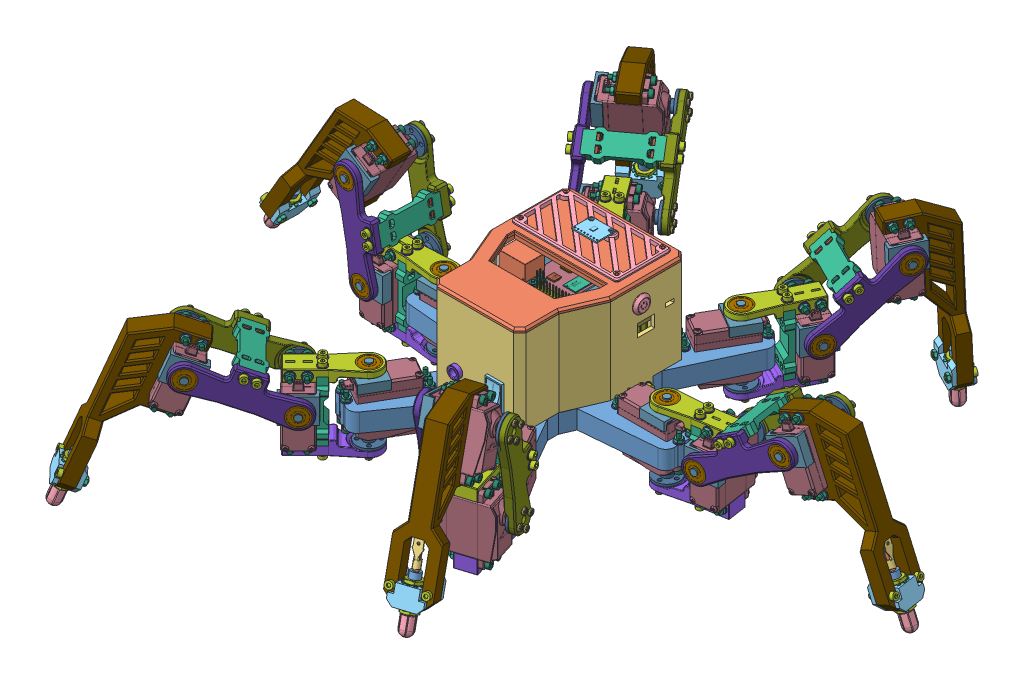
SolidWorks assembly HEXUMI_DSSERVO, configuration Default. Lengths in mm. (continued)
Mates (geometry in assembly coordinates): (continued)
- Concentric24: concentric aligned: cylinder of M3_WASHER-16 through (-104.9 0.5 30.3) axis (0 -1 0) radius 1.6; cylinder of M3_HEX_NUT-23 through (-104.9 2.9 30.3) axis (0 -1 0) radius 1.5
- Concentric25: concentric aligned: cylinder of M3_WASHER-15 through (-55.3 0.5 20.3) axis (0 -1 0) radius 1.6; cylinder of M3_HEX_NUT-20 through (-55.3 2.9 20.3) axis (0 -1 0) radius 1.5
- Coincident21: coincident anti-aligned: plane of M3_WASHER-15 through (-55.3 0.5 20.3) normal (0 1 0); plane of M3_HEX_NUT-20 through (-55.3 0.5 20.3) normal (0 -1 0)
- Coincident22: coincident anti-aligned: plane of M3_WASHER-17 through (-66.6069 0.5 -80.2666) normal (0 1 0); plane of M3_HEX_NUT-22 through (-66.6069 0.5 -80.2666) normal (0 -1 0)
- Coincident23: coincident anti-aligned: plane of M3_WASHER-16 through (-104.9 0.5 30.3) normal (0 1 0); plane of M3_HEX_NUT-23 through (-104.9 0.5 30.3) normal (0 -1 0)
- Concentric26: concentric aligned: circle of M3_WASHER-13; circle of M3_HEX_NUT-16
- Coincident24: coincident anti-aligned: plane of M3_WASHER-13 through (-33.1467 0.5 -42.3117) normal (0 1 0); plane of M3_HEX_NUT-16 through (-33.1467 0.5 -42.3117) normal (0 -1 0)
- Coincident25: coincident anti-aligned: plane of M3_WASHER-11 through (-41.8069 0.5 -37.3117) normal (0 1 0); plane of M3_HEX_NUT-10 through (-41.8069 0.5 -37.3117) normal (0 -1 0)
- Coincident26: coincident anti-aligned: plane of M3_WASHER-12 through (-57.9467 0.5 -85.2666) normal (0 1 0); plane of M3_HEX_NUT-21 through (-57.9467 0.5 -85.2666) normal (0 -1 0)
- Coincident27: coincident anti-aligned: plane of M3_WASHER-14 through (-55.3 0.5 30.3) normal (0 1 0); plane of M3_HEX_NUT-19 through (-55.3 0.5 30.3) normal (0 -1 0)
- Coincident29: coincident anti-aligned: plane of M3_WASHER-8 through (-66.9533 0.5 131.0666) normal (0 1 0); plane of M3_HEX_NUT-9 through (-66.9533 0.5 131.0666) normal (0 -1 0)
- Coincident30: coincident anti-aligned: plane of M3_WASHER-9 through (33.1467 0.5 -42.3117) normal (0 1 0); plane of M3_HEX_NUT-8 through (33.1467 0.5 -42.3117) normal (0 -1 0)
- Coincident31: coincident anti-aligned: plane of M3_WASHER-5 through (41.8069 0.5 -37.3117) normal (0 1 0); plane of M3_HEX_NUT-14 through (41.8069 0.5 -37.3117) normal (0 -1 0)
- Coincident32: coincident anti-aligned: plane of M3_WASHER-6 through (-42.1533 0.5 88.1117) normal (0 1 0); plane of M3_HEX_NUT-15 through (-42.1533 0.5 88.1117) normal (0 -1 0)
- Coincident33: coincident anti-aligned: plane of M3_WASHER-1 through (-58.2931 0.5 136.0666) normal (0 1 0); plane of M3_HEX_NUT-24 through (-58.2931 0.5 136.0666) normal (0 -1 0)
- Coincident34: coincident anti-aligned: plane of M3_WASHER-23 through (66.6069 0.5 -80.2666) normal (0 1 0); plane of M3_HEX_NUT-18 through (66.6069 0.5 -80.2666) normal (0 -1 0)
- Coincident35: coincident anti-aligned: plane of M3_WASHER-22 through (57.9467 0.5 -85.2666) normal (0 1 0); plane of M3_HEX_NUT-11 through (57.9467 0.5 -85.2666) normal (0 -1 0)
- Coincident36: coincident anti-aligned: plane of M3_WASHER-21 through (58.2931 0.5 136.0666) normal (0 1 0); plane of M3_HEX_NUT-4 through (58.2931 0.5 136.0666) normal (0 -1 0)
- Coincident37: coincident anti-aligned: plane of M3_WASHER-20 through (66.9533 0.5 131.0666) normal (0 1 0); plane of M3_HEX_NUT-17 through (66.9533 0.5 131.0666) normal (0 -1 0)
- Coincident38: coincident anti-aligned: plane of M3_WASHER-18 through (104.9 0.5 20.3) normal (0 1 0); plane of M3_HEX_NUT-2 through (104.9 0.5 20.3) normal (0 -1 0)
- Coincident39: coincident anti-aligned: plane of M3_WASHER-19 through (33.4931 0.5 93.1117) normal (0 1 0); plane of M3_HEX_NUT-3 through (33.4931 0.5 93.1117) normal (0 -1 0)
- Coincident40: coincident anti-aligned: plane of M3_WASHER-7 through (55.3 0.5 30.3) normal (0 1 0); plane of M3_HEX_NUT-7 through (55.3 0.5 30.3) normal (0 -1 0)
- Coincident41: coincident anti-aligned: plane of M3_WASHER-2 through (42.1533 0.5 88.1117) normal (0 1 0); plane of M3_HEX_NUT-5 through (42.1533 0.5 88.1117) normal (0 -1 0)
- Coincident42: coincident anti-aligned: plane of M3_WASHER-3 through (104.9 0.5 30.3) normal (0 1 0); plane of M3_HEX_NUT-6 through (104.9 0.5 30.3) normal (0 -1 0)
- Coincident43: coincident anti-aligned: plane of M3_WASHER-4 through (55.3 0.5 20.3) normal (0 1 0); plane of M3_HEX_NUT-13 through (55.3 0.5 20.3) normal (0 -1 0)
- Coincident44: coincident anti-aligned: plane of M3_WASHER-10 through (-33.4931 0.5 93.1117) normal (0 1 0); plane of M3_HEX_NUT-12 through (-33.4931 0.5 93.1117) normal (0 -1 0)
- Concentric27: concentric aligned: cylinder of BODY_ASM-1/MAIN_FRAME-1 through (-104.9 0 30.3) axis (0 -1 0) radius 1.5; cylinder of M3_STEEL_HEX_BOLT-20 through (-104.9 6.8 30.3) axis (0 -1 0) radius 1.5
- Concentric28: concentric aligned: cylinder of BODY_ASM-1/MAIN_FRAME-1 through (-104.9 0 20.3) axis (0 -1 0) radius 1.5; cylinder of M3_STEEL_HEX_BOLT-19 through (-104.9 6.8 20.3) axis (0 -1 0) radius 1.5
- Concentric29: concentric aligned: cylinder of BODY_ASM-1/MAIN_FRAME-1 through (-57.9467 0 -85.2666) axis (0 -1 0) radius 1.5; cylinder of M3_STEEL_HEX_BOLT-18 through (-57.9467 6.8 -85.2666) axis (0 -1 0) radius 1.5
- Concentric30: concentric aligned: cylinder of BODY_ASM-1/MAIN_FRAME-1 through (-66.6069 0 -80.2666) axis (0 -1 0) radius 1.5; cylinder of M3_STEEL_HEX_BOLT-17 through (-66.6069 6.8 -80.2666) axis (0 -1 0) radius 1.5
- Concentric31: concentric aligned: cylinder of BODY_ASM-1/MAIN_FRAME-1 through (57.9467 0 -85.2666) axis (0 -1 0) radius 1.5; cylinder of M3_STEEL_HEX_BOLT-16 through (57.9467 6.8 -85.2666) axis (0 -1 0) radius 1.5
- Concentric32: concentric aligned: cylinder of BODY_ASM-1/MAIN_FRAME-1 through (66.6069 0 -80.2666) axis (0 -1 0) radius 1.5; cylinder of M3_STEEL_HEX_BOLT-15 through (66.6069 6.8 -80.2666) axis (0 -1 0) radius 1.5
- Concentric33: concentric aligned: cylinder of BODY_ASM-1/MAIN_FRAME-1 through (104.9 0 30.3) axis (0 -1 0) radius 1.5; cylinder of M3_STEEL_HEX_BOLT-2 through (104.9 6.8 30.3) axis (0 -1 0) radius 1.5
- Concentric34: concentric aligned: cylinder of BODY_ASM-1/MAIN_FRAME-1 through (104.9 0 20.3) axis (0 -1 0) radius 1.5; cylinder of M3_STEEL_HEX_BOLT-14 through (104.9 6.8 20.3) axis (0 -1 0) radius 1.5
- Concentric35: concentric aligned: cylinder of BODY_ASM-1/MAIN_FRAME-1 through (66.9533 0 131.0666) axis (0 -1 0) radius 1.5; cylinder of M3_STEEL_HEX_BOLT-1 through (66.9533 6.8 131.0666) axis (0 -1 0) radius 1.5
- Concentric36: concentric aligned: cylinder of BODY_ASM-1/MAIN_FRAME-1 through (58.2931 0 136.0666) axis (0 -1 0) radius 1.5; cylinder of M3_STEEL_HEX_BOLT-24 through (58.2931 6.8 136.0666) axis (0 -1 0) radius 1.5
- Concentric37: concentric aligned: cylinder of BODY_ASM-1/MAIN_FRAME-1 through (-58.2931 0 136.0666) axis (0 -1 0) radius 1.5; cylinder of M3_STEEL_HEX_BOLT-3 through (-58.2931 6.8 136.0666) axis (0 -1 0) radius 1.5
- Concentric38: concentric aligned: cylinder of BODY_ASM-1/MAIN_FRAME-1 through (-66.9533 0 131.0666) axis (0 -1 0) radius 1.5; cylinder of M3_STEEL_HEX_BOLT-21 through (-66.9533 6.8 131.0666) axis (0 -1 0) radius 1.5
- Concentric39: concentric aligned: cylinder of BODY_ASM-1/MAIN_FRAME-1 through (-42.1533 0 88.1117) axis (0 -1 0) radius 1.5; cylinder of M3_STEEL_HEX_BOLT-13 through (-42.1533 6.8 88.1117) axis (0 -1 0) radius 1.5
- Concentric40: concentric aligned: cylinder of BODY_ASM-1/MAIN_FRAME-1 through (-33.4931 0 93.1117) axis (0 -1 0) radius 1.5; cylinder of M3_STEEL_HEX_BOLT-12 through (-33.4931 6.8 93.1117) axis (0 -1 0) radius 1.5
- Concentric41: concentric aligned: cylinder of BODY_ASM-1/MAIN_FRAME-1 through (-55.3 0 30.3) axis (0 -1 0) radius 1.5; cylinder of M3_STEEL_HEX_BOLT-11 through (-55.3 6.8 30.3) axis (0 -1 0) radius 1.5
- Concentric42: concentric aligned: cylinder of BODY_ASM-1/MAIN_FRAME-1 through (-55.3 0 20.3) axis (0 -1 0) radius 1.5; cylinder of M3_STEEL_HEX_BOLT-10 through (-55.3 6.8 20.3) axis (0 -1 0) radius 1.5
- Concentric43: concentric aligned: cylinder of BODY_ASM-1/MAIN_FRAME-1 through (33.4931 0 93.1117) axis (0 -1 0) radius 1.5; cylinder of M3_STEEL_HEX_BOLT-9 through (33.4931 6.8 93.1117) axis (0 -1 0) radius 1.5
- Concentric44: concentric aligned: cylinder of BODY_ASM-1/MAIN_FRAME-1 through (42.1533 0 88.1117) axis (0 -1 0) radius 1.5; cylinder of M3_STEEL_HEX_BOLT-8 through (42.1533 6.8 88.1117) axis (0 -1 0) radius 1.5
- Concentric45: concentric aligned: cylinder of BODY_ASM-1/MAIN_FRAME-1 through (55.3 0 30.3) axis (0 -1 0) radius 1.5; cylinder of M3_STEEL_HEX_BOLT-7 through (55.3 6.8 30.3) axis (0 -1 0) radius 1.5
- Concentric46: concentric aligned: cylinder of BODY_ASM-1/MAIN_FRAME-1 through (55.3 0 20.3) axis (0 -1 0) radius 1.5; cylinder of M3_STEEL_HEX_BOLT-6 through (55.3 6.8 20.3) axis (0 -1 0) radius 1.5
- Concentric47: concentric aligned: cylinder of BODY_ASM-1/MAIN_FRAME-1 through (41.8069 0 -37.3117) axis (0 -1 0) radius 1.5; cylinder of M3_STEEL_HEX_BOLT-5 through (41.8069 6.8 -37.3117) axis (0 -1 0) radius 1.5
- Concentric48: concentric aligned: cylinder of BODY_ASM-1/MAIN_FRAME-1 through (33.1467 0 -42.3117) axis (0 -1 0) radius 1.5; cylinder of M3_STEEL_HEX_BOLT-23 through (33.1467 6.8 -42.3117) axis (0 -1 0) radius 1.5
- Concentric49: concentric aligned: cylinder of BODY_ASM-1/MAIN_FRAME-1 through (-33.1467 0 -42.3117) axis (0 -1 0) radius 1.5; cylinder of M3_STEEL_HEX_BOLT-22 through (-33.1467 6.8 -42.3117) axis (0 -1 0) radius 1.5
- Concentric50: concentric aligned: cylinder of BODY_ASM-1/MAIN_FRAME-1 through (-41.8069 0 -37.3117) axis (0 -1 0) radius 1.5; cylinder of M3_STEEL_HEX_BOLT-4 through (-41.8069 6.8 -37.3117) axis (0 -1 0) radius 1.5
- Coincident46: coincident anti-aligned: plane of LEG_L-1/SERVO_ASM-2/SW2020 DS3225MG Servo 25Kg 4.8-6.8V-2 through (-54.8768 -18.2 -69.9494) normal (0 -1 0); plane of M3_STEEL_HEX_BOLT-4 through (-41.8069 -18.2 -37.3117) normal (0 1 0)
- Coincident47: coincident anti-aligned: plane of LEG_L-1/SERVO_ASM-2/SW2020 DS3225MG Servo 25Kg 4.8-6.8V-2 through (-54.8768 -18.2 -69.9494) normal (0 -1 0); plane of M3_STEEL_HEX_BOLT-22 through (-33.1467 -18.2 -42.3117) normal (0 1 0)
- Coincident48: coincident anti-aligned: plane of LEG_L-3/SERVO_ASM-2/SW2020 DS3225MG Servo 25Kg 4.8-6.8V-2 through (-90.1 -18.2 25.3) normal (0 -1 0); plane of M3_STEEL_HEX_BOLT-10 through (-55.3 -18.2 20.3) normal (0 1 0)
- Coincident49: coincident anti-aligned: plane of LEG_L-1/SERVO_ASM-2/SW2020 DS3225MG Servo 25Kg 4.8-6.8V-2 through (-54.8768 -18.2 -69.9494) normal (0 -1 0); plane of M3_STEEL_HEX_BOLT-18 through (-57.9467 -18.2 -85.2666) normal (0 1 0)
- Coincident50: coincident anti-aligned: plane of LEG_L-1/SERVO_ASM-2/SW2020 DS3225MG Servo 25Kg 4.8-6.8V-2 through (-54.8768 -18.2 -69.9494) normal (0 -1 0); plane of M3_STEEL_HEX_BOLT-17 through (-66.6069 -18.2 -80.2666) normal (0 1 0)
- Coincident51: coincident anti-aligned: plane of LEG_L-3/SERVO_ASM-2/SW2020 DS3225MG Servo 25Kg 4.8-6.8V-2 through (-90.1 -18.2 25.3) normal (0 -1 0); plane of M3_STEEL_HEX_BOLT-20 through (-104.9 -18.2 30.3) normal (0 1 0)
- Coincident52: coincident anti-aligned: plane of LEG_L-3/SERVO_ASM-2/SW2020 DS3225MG Servo 25Kg 4.8-6.8V-2 through (-90.1 -18.2 25.3) normal (0 -1 0); plane of M3_STEEL_HEX_BOLT-19 through (-104.9 -18.2 20.3) normal (0 1 0)
- Coincident53: coincident anti-aligned: plane of LEG_L-2/SERVO_ASM-2/SW2020 DS3225MG Servo 25Kg 4.8-6.8V-2 through (-55.2232 -18.2 120.7494) normal (0 -1 0); plane of M3_STEEL_HEX_BOLT-3 through (-58.2931 -18.2 136.0666) normal (0 1 0)
- Coincident54: coincident anti-aligned: plane of LEG_L-2/SERVO_ASM-2/SW2020 DS3225MG Servo 25Kg 4.8-6.8V-2 through (-55.2232 -18.2 120.7494) normal (0 -1 0); plane of M3_STEEL_HEX_BOLT-21 through (-66.9533 -18.2 131.0666) normal (0 1 0)
- Coincident55: coincident anti-aligned: plane of LEG_R-2/SERVO_ASM-2/SW2020 DS3225MG Servo 25Kg 4.8-6.8V-2 through (55.2232 -18.2 120.7494) normal (0 -1 0); plane of M3_STEEL_HEX_BOLT-1 through (66.9533 -18.2 131.0666) normal (0 1 0)
- Coincident56: coincident anti-aligned: plane of LEG_R-2/SERVO_ASM-2/SW2020 DS3225MG Servo 25Kg 4.8-6.8V-2 through (55.2232 -18.2 120.7494) normal (0 -1 0); plane of M3_STEEL_HEX_BOLT-24 through (58.2931 -18.2 136.0666) normal (0 1 0)
- Coincident57: coincident anti-aligned: plane of LEG_R-1/SERVO_ASM-2/SW2020 DS3225MG Servo 25Kg 4.8-6.8V-2 through (90.1 -18.2 25.3) normal (0 -1 0); plane of M3_STEEL_HEX_BOLT-14 through (104.9 -18.2 20.3) normal (0 1 0)
- Coincident58: coincident anti-aligned: plane of LEG_R-1/SERVO_ASM-2/SW2020 DS3225MG Servo 25Kg 4.8-6.8V-2 through (90.1 -18.2 25.3) normal (0 -1 0); plane of M3_STEEL_HEX_BOLT-2 through (104.9 -18.2 30.3) normal (0 1 0)
- Coincident59: coincident anti-aligned: plane of LEG_R-3/SERVO_ASM-2/SW2020 DS3225MG Servo 25Kg 4.8-6.8V-2 through (54.8768 -18.2 -69.9494) normal (0 -1 0); plane of M3_STEEL_HEX_BOLT-16 through (57.9467 -18.2 -85.2666) normal (0 1 0)
- Coincident60: coincident anti-aligned: plane of LEG_R-3/SERVO_ASM-2/SW2020 DS3225MG Servo 25Kg 4.8-6.8V-2 through (54.8768 -18.2 -69.9494) normal (0 -1 0); plane of M3_STEEL_HEX_BOLT-15 through (66.6069 -18.2 -80.2666) normal (0 1 0)
- Coincident61: coincident anti-aligned: plane of LEG_L-3/SERVO_ASM-2/SW2020 DS3225MG Servo 25Kg 4.8-6.8V-2 through (-90.1 -18.2 25.3) normal (0 -1 0); plane of M3_STEEL_HEX_BOLT-11 through (-55.3 -18.2 30.3) normal (0 1 0)
- Coincident62: coincident anti-aligned: plane of LEG_L-2/SERVO_ASM-2/SW2020 DS3225MG Servo 25Kg 4.8-6.8V-2 through (-55.2232 -18.2 120.7494) normal (0 -1 0); plane of M3_STEEL_HEX_BOLT-12 through (-33.4931 -18.2 93.1117) normal (0 1 0)
- Coincident63: coincident anti-aligned: plane of LEG_L-2/SERVO_ASM-2/SW2020 DS3225MG Servo 25Kg 4.8-6.8V-2 through (-55.2232 -18.2 120.7494) normal (0 -1 0); circle of M3_STEEL_HEX_BOLT-13
- Coincident64: coincident anti-aligned: plane of LEG_R-2/SERVO_ASM-2/SW2020 DS3225MG Servo 25Kg 4.8-6.8V-2 through (55.2232 -18.2 120.7494) normal (0 -1 0); plane of M3_STEEL_HEX_BOLT-8 through (42.1533 -18.2 88.1117) normal (0 1 0)
- Coincident65: coincident anti-aligned: plane of LEG_R-2/SERVO_ASM-2/SW2020 DS3225MG Servo 25Kg 4.8-6.8V-2 through (55.2232 -18.2 120.7494) normal (0 -1 0); plane of M3_STEEL_HEX_BOLT-9 through (33.4931 -18.2 93.1117) normal (0 1 0)
- Coincident66: coincident anti-aligned: plane of LEG_R-1/SERVO_ASM-2/SW2020 DS3225MG Servo 25Kg 4.8-6.8V-2 through (90.1 -18.2 25.3) normal (0 -1 0); plane of M3_STEEL_HEX_BOLT-6 through (55.3 -18.2 20.3) normal (0 1 0)
- Coincident67: coincident anti-aligned: plane of LEG_R-1/SERVO_ASM-2/SW2020 DS3225MG Servo 25Kg 4.8-6.8V-2 through (90.1 -18.2 25.3) normal (0 -1 0); plane of M3_STEEL_HEX_BOLT-7 through (55.3 -18.2 30.3) normal (0 1 0)
- Coincident68: coincident anti-aligned: plane of LEG_R-3/SERVO_ASM-2/SW2020 DS3225MG Servo 25Kg 4.8-6.8V-2 through (54.8768 -18.2 -69.9494) normal (0 -1 0); plane of M3_STEEL_HEX_BOLT-5 through (41.8069 -18.2 -37.3117) normal (0 1 0)
- Coincident69: coincident anti-aligned: plane of LEG_R-3/SERVO_ASM-2/SW2020 DS3225MG Servo 25Kg 4.8-6.8V-2 through (54.8768 -18.2 -69.9494) normal (0 -1 0); plane of M3_STEEL_HEX_BOLT-23 through (33.1467 -18.2 -42.3117) normal (0 1 0)
- Concentric51: concentric aligned: cylinder of M3_STEEL_HEX_BOLT-10 through (-55.3 -18.2 20.3) axis (0 -1 0) radius 2.84; cylinder of M3_HEX_NUT-20 through (-55.3 2.9 20.3) axis (0 -1 0) radius 1.5
- Concentric52: concentric aligned: cylinder of M3_STEEL_HEX_BOLT-11 through (-55.3 -18.2 30.3) axis (0 -1 0) radius 2.84; cylinder of M3_HEX_NUT-19 through (-55.3 2.9 30.3) axis (0 -1 0) radius 1.5
- Concentric53: concentric aligned: cylinder of M3_STEEL_HEX_BOLT-22 through (-33.1467 -18.2 -42.3117) axis (0 -1 0) radius 2.84; cylinder of M3_HEX_NUT-16 through (-33.1467 2.9 -42.3117) axis (0 -1 0) radius 1.5
- Concentric54: concentric aligned: cylinder of M3_STEEL_HEX_BOLT-4 through (-41.8069 -18.2 -37.3117) axis (0 -1 0) radius 2.84; cylinder of M3_HEX_NUT-10 through (-41.8069 2.9 -37.3117) axis (0 -1 0) radius 1.5
- Concentric55: concentric aligned: cylinder of M3_STEEL_HEX_BOLT-18 through (-57.9467 -18.2 -85.2666) axis (0 -1 0) radius 2.84; cylinder of M3_HEX_NUT-21 through (-57.9467 2.9 -85.2666) axis (0 -1 0) radius 1.5
- Concentric56: concentric aligned: cylinder of M3_STEEL_HEX_BOLT-17 through (-66.6069 -18.2 -80.2666) axis (0 -1 0) radius 2.84; cylinder of M3_HEX_NUT-22 through (-66.6069 2.9 -80.2666) axis (0 -1 0) radius 1.5
- Concentric57: concentric aligned: cylinder of M3_STEEL_HEX_BOLT-20 through (-104.9 -18.2 30.3) axis (0 -1 0) radius 2.84; cylinder of M3_HEX_NUT-23 through (-104.9 2.9 30.3) axis (0 -1 0) radius 1.5
- Concentric58: concentric aligned: cylinder of M3_STEEL_HEX_BOLT-5 through (41.8069 -18.2 -37.3117) axis (0 -1 0) radius 2.84; cylinder of M3_HEX_NUT-14 through (41.8069 2.9 -37.3117) axis (0 -1 0) radius 1.5
- Concentric59: concentric aligned: cylinder of M3_STEEL_HEX_BOLT-23 through (33.1467 -18.2 -42.3117) axis (0 -1 0) radius 2.84; cylinder of M3_HEX_NUT-8 through (33.1467 2.9 -42.3117) axis (0 -1 0) radius 1.5
- Concentric62: concentric aligned: cylinder of M3_STEEL_HEX_BOLT-13 through (-42.1533 -18.2 88.1117) axis (0 -1 0) radius 2.84; cylinder of M3_HEX_NUT-15 through (-42.1533 2.9 88.1117) axis (0 -1 0) radius 1.5
- Concentric63: concentric aligned: cylinder of M3_STEEL_HEX_BOLT-21 through (-66.9533 -18.2 131.0666) axis (0 -1 0) radius 2.84; cylinder of M3_HEX_NUT-9 through (-66.9533 2.9 131.0666) axis (0 -1 0) radius 1.5
- Concentric64: concentric aligned: cylinder of M3_STEEL_HEX_BOLT-3 through (-58.2931 -18.2 136.0666) axis (0 -1 0) radius 2.84; cylinder of M3_HEX_NUT-24 through (-58.2931 2.9 136.0666) axis (0 -1 0) radius 1.5
- Concentric66: concentric aligned: cylinder of M3_STEEL_HEX_BOLT-7 through (55.3 -18.2 30.3) axis (0 -1 0) radius 2.84; cylinder of M3_HEX_NUT-7 through (55.3 2.9 30.3) axis (0 -1 0) radius 1.5
- Concentric67: concentric aligned: cylinder of M3_STEEL_HEX_BOLT-6 through (55.3 -18.2 20.3) axis (0 -1 0) radius 2.84; cylinder of M3_HEX_NUT-13 through (55.3 2.9 20.3) axis (0 -1 0) radius 1.5
- Concentric68: concentric aligned: cylinder of M3_STEEL_HEX_BOLT-2 through (104.9 -18.2 30.3) axis (0 -1 0) radius 2.84; cylinder of M3_HEX_NUT-6 through (104.9 2.9 30.3) axis (0 -1 0) radius 1.5
- Concentric69: concentric aligned: cylinder of M3_STEEL_HEX_BOLT-14 through (104.9 -18.2 20.3) axis (0 -1 0) radius 2.84; cylinder of M3_HEX_NUT-2 through (104.9 2.9 20.3) axis (0 -1 0) radius 1.5
- Parallel1: parallel aligned: cylinder of M3_STEEL_HEX_BOLT-15 through (66.6069 -18.2 -80.2666) axis (0 -1 0) radius 2.84; cylinder of M3_HEX_NUT-16 through (-33.1467 2.9 -42.3117) axis (0 -1 0) radius 1.5
- Coincident70: coincident anti-aligned: plane of BODY_ASM-1/MAIN_FRAME-1 through (34 0 55.6123) normal (0 1 0); plane of M3_WASHER-6 through (-42.1533 0 88.1117) normal (0 -1 0)
- Coincident71: coincident anti-aligned: plane of BODY_ASM-1/MAIN_FRAME-1 through (34 0 55.6123) normal (0 1 0); plane of M3_WASHER-14 through (-55.3 0 30.3) normal (0 -1 0)
- Coincident72: coincident anti-aligned: plane of BODY_ASM-1/MAIN_FRAME-1 through (34 0 55.6123) normal (0 1 0); plane of M3_WASHER-15 through (-55.3 0 20.3) normal (0 -1 0)
- Coincident73: coincident anti-aligned: plane of BODY_ASM-1/MAIN_FRAME-1 through (34 0 55.6123) normal (0 1 0); plane of M3_WASHER-11 through (-41.8069 0 -37.3117) normal (0 -1 0)
- Coincident74: coincident anti-aligned: plane of BODY_ASM-1/MAIN_FRAME-1 through (34 0 55.6123) normal (0 1 0); plane of M3_WASHER-12 through (-57.9467 0 -85.2666) normal (0 -1 0)
- Coincident75: coincident anti-aligned: plane of BODY_ASM-1/MAIN_FRAME-1 through (34 0 55.6123) normal (0 1 0); plane of M3_WASHER-17 through (-66.6069 0 -80.2666) normal (0 -1 0)
- Coincident76: coincident anti-aligned: plane of BODY_ASM-1/MAIN_FRAME-1 through (34 0 55.6123) normal (0 1 0); plane of M3_WASHER-9 through (33.1467 0 -42.3117) normal (0 -1 0)
- Coincident77: coincident anti-aligned: plane of BODY_ASM-1/MAIN_FRAME-1 through (34 0 55.6123) normal (0 1 0); plane of M3_WASHER-5 through (41.8069 0 -37.3117) normal (0 -1 0)
- Coincident79: coincident anti-aligned: plane of BODY_ASM-1/MAIN_FRAME-1 through (34 0 55.6123) normal (0 1 0); plane of M3_WASHER-7 through (55.3 0 30.3) normal (0 -1 0)
- Coincident80: coincident anti-aligned: plane of BODY_ASM-1/MAIN_FRAME-1 through (34 0 55.6123) normal (0 1 0); plane of M3_WASHER-4 through (55.3 0 20.3) normal (0 -1 0)
- Coincident81: coincident anti-aligned: plane of BODY_ASM-1/MAIN_FRAME-1 through (34 0 55.6123) normal (0 1 0); plane of M3_WASHER-3 through (104.9 0 30.3) normal (0 -1 0)
- Coincident82: coincident anti-aligned: plane of BODY_ASM-1/MAIN_FRAME-1 through (34 0 55.6123) normal (0 1 0); plane of M3_WASHER-18 through (104.9 0 20.3) normal (0 -1 0)
- Coincident83: coincident anti-aligned: plane of BODY_ASM-1/MAIN_FRAME-1 through (34 0 55.6123) normal (0 1 0); plane of M3_WASHER-1 through (-58.2931 0 136.0666) normal (0 -1 0)
- Coincident84: coincident anti-aligned: plane of BODY_ASM-1/MAIN_FRAME-1 through (34 0 55.6123) normal (0 1 0); plane of M3_WASHER-8 through (-66.9533 0 131.0666) normal (0 -1 0)
- Coincident85: coincident anti-aligned: plane of BODY_ASM-1/MAIN_FRAME-1 through (34 0 55.6123) normal (0 1 0); plane of M3_WASHER-16 through (-104.9 0 30.3) normal (0 -1 0)
- Concentric71: concentric aligned: cylinder of M3_STEEL_HEX_BOLT-12 through (-33.4931 6.8 93.1117) axis (0 -1 0) radius 1.5; cylinder of M3_HEX_NUT-12 through (-33.4931 2.9 93.1117) axis (0 -1 0) radius 1.5
- Coincident86: coincident anti-aligned: plane of BODY_ASM-1/MAIN_FRAME-1 through (34 0 55.6123) normal (0 1 0); plane of M3_WASHER-10 through (-33.4931 0 93.1117) normal (0 -1 0)
- Concentric76: concentric aligned: cylinder of M3_STEEL_HEX_BOLT-8 through (42.1533 6.8 88.1117) axis (0 -1 0) radius 1.5; cylinder of M3_HEX_NUT-5 through (42.1533 2.9 88.1117) axis (0 -1 0) radius 1.5
- Concentric77: concentric aligned: cylinder of M3_STEEL_HEX_BOLT-8 through (42.1533 -18.2 88.1117) axis (0 -1 0) radius 2.84; cylinder of M3_HEX_NUT-5 through (42.1533 2.9 88.1117) axis (0 -1 0) radius 1.5
- Concentric79: concentric aligned: cylinder of M3_STEEL_HEX_BOLT-22 through (-33.1467 6.8 -42.3117) axis (0 -1 0) radius 1.5; cylinder of M3_HEX_NUT-16 through (-33.1467 2.9 -42.3117) axis (0 -1 0) radius 1.5
- Coincident87: coincident anti-aligned: plane of BODY_ASM-1/MAIN_FRAME-1 through (34 0 55.6123) normal (0 1 0); plane of M3_WASHER-13 through (-33.1467 0 -42.3117) normal (0 -1 0)
- Concentric80: concentric aligned: cylinder of M3_STEEL_HEX_BOLT-9 through (33.4931 6.8 93.1117) axis (0 -1 0) radius 1.5; cylinder of M3_HEX_NUT-3 through (33.4931 2.9 93.1117) axis (0 -1 0) radius 1.5
- Coincident88: coincident anti-aligned: plane of BODY_ASM-1/MAIN_FRAME-1 through (34 0 55.6123) normal (0 1 0); plane of M3_WASHER-19 through (33.4931 0 93.1117) normal (0 -1 0)
- Concentric81: concentric aligned: cylinder of M3_STEEL_HEX_BOLT-15 through (66.6069 6.8 -80.2666) axis (0 -1 0) radius 1.5; cylinder of M3_HEX_NUT-18 through (66.6069 2.9 -80.2666) axis (0 -1 0) radius 1.5
- Coincident89: coincident anti-aligned: plane of BODY_ASM-1/MAIN_FRAME-1 through (34 0 55.6123) normal (0 1 0); plane of M3_WASHER-23 through (66.6069 0 -80.2666) normal (0 -1 0)
- Concentric82: concentric aligned: cylinder of M3_STEEL_HEX_BOLT-1 through (66.9533 6.8 131.0666) axis (0 -1 0) radius 1.5; cylinder of M3_HEX_NUT-17 through (66.9533 2.9 131.0666) axis (0 -1 0) radius 1.5
- Coincident90: coincident anti-aligned: plane of BODY_ASM-1/MAIN_FRAME-1 through (34 0 55.6123) normal (0 1 0); plane of M3_WASHER-20 through (66.9533 0 131.0666) normal (0 -1 0)
- Concentric84: concentric aligned: cylinder of M3_STEEL_HEX_BOLT-24 through (58.2931 6.8 136.0666) axis (0 -1 0) radius 1.5; cylinder of M3_HEX_NUT-4 through (58.2931 2.9 136.0666) axis (0 -1 0) radius 1.5
- Coincident91: coincident anti-aligned: plane of BODY_ASM-1/MAIN_FRAME-1 through (34 0 55.6123) normal (0 1 0); plane of M3_WASHER-21 through (58.2931 0 136.0666) normal (0 -1 0)
- Concentric85: concentric aligned: cylinder of M3_STEEL_HEX_BOLT-16 through (57.9467 6.8 -85.2666) axis (0 -1 0) radius 1.5; cylinder of M3_HEX_NUT-11 through (57.9467 2.9 -85.2666) axis (0 -1 0) radius 1.5
- Coincident92: coincident anti-aligned: plane of BODY_ASM-1/MAIN_FRAME-1 through (34 0 55.6123) normal (0 1 0); plane of M3_WASHER-22 through (57.9467 0 -85.2666) normal (0 -1 0)
- Coincident93: coincident anti-aligned: plane of BODY_ASM-1/MAIN_FRAME-1 through (34 0 55.6123) normal (0 1 0); plane of M3_WASHER-2 through (42.1533 0 88.1117) normal (0 -1 0)
- Concentric86: concentric aligned: cylinder of M3_WASHER-25 through (-104.9 0 20.3) axis (0 1 0) radius 1.6; cylinder of M3_HEX_NUT-25 through (-104.9 0.5 20.3) axis (0 1 0) radius 1.5
- Coincident94: coincident anti-aligned: plane of M3_WASHER-25 through (-104.9 0.5 20.3) normal (0 1 0); plane of M3_HEX_NUT-25 through (-104.9 0.5 20.3) normal (0 -1 0)
- Concentric87: concentric anti-aligned: cylinder of M3_STEEL_HEX_BOLT-19 through (-104.9 6.8 20.3) axis (0 -1 0) radius 1.5; cylinder of M3_HEX_NUT-25 through (-104.9 0.5 20.3) axis (0 1 0) radius 1.5
- Coincident95: coincident anti-aligned: plane of BODY_ASM-1/MAIN_FRAME-1 through (34 0 55.6123) normal (0 1 0); plane of M3_WASHER-25 through (-104.9 0 20.3) normal (0 -1 0)
- Concentric91: concentric aligned: cylinder of BODY_ASM-1/MID CASE-1 through (-15 19.5 -33.001) axis (0 0 1) radius 3.75; cylinder of DC_PLUG-1 through (-15 19.5 84.5) axis (0 0 1) radius 3.65
- Coincident97: coincident anti-aligned: plane of BODY_ASM-1/MID CASE-1 through (36 69 90) normal (0 0 1); plane of DC_PLUG-1 through (-15 19.5 90) normal (0 0 -1)
